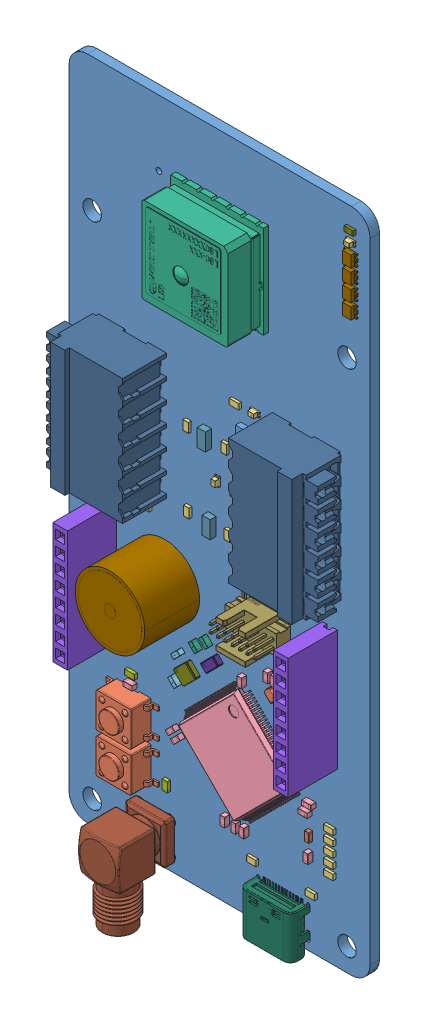
SolidWorks assembly Main_Board_1_1, configuration Default. Lengths in mm.
Overall size (70 133 15.95).
128 component instances, 40 part files, 0 mates.
Components (placement in the parent):
- Main_Board_1_1_BOARD-1: Main_Board_1_1_BOARD [Default] at origin size (52 115 1.63)
- BMP581_CMP-048-000000-2-1: BMP581_CMP-048-000000-2 [Default] at (43 50.5 0.0203) x (-0.707107 -0.707107 0) z (0 0 -1) size (2 2 0.8)
- BMP581_CMP-048-000000-2-2: BMP581_CMP-048-000000-2 [Default] at (45.5 45.5 1.6065) x (0.707107 -0.707107 0) z (0 0 1) size (2 2 0.8)
- RESC1609X50X30ML8T20_CMP-009-00185-4-1: RESC1609X50X30ML8T20_CMP-009-00185-4 [Default] at (40.25 53.25 0.0203) x (0 1 0) z (0 0 -1) size (1.65 0.95 0.5)
- RESC1609X50X30ML8T20_CMP-009-00185-4-2: RESC1609X50X30ML8T20_CMP-009-00185-4 [Default] at (47.5 49 0.0203) x (0 1 0) z (0 0 -1) size (1.65 0.95 0.5)
- RESC1609X50X30ML8T20_CMP-009-00185-4-3: RESC1609X50X30ML8T20_CMP-009-00185-4 [Default] at (41.5 53.25 0.0203) x (0 1 0) z (0 0 -1) size (1.65 0.95 0.5)
- RESC1609X50X30ML8T20_CMP-009-00185-4-4: RESC1609X50X30ML8T20_CMP-009-00185-4 [Default] at (46.0298 49.0299 0.0203) x (0 1 0) z (0 0 -1) size (1.65 0.95 0.5)
- RESC1609X50X30ML8T20_CMP-009-00185-4-5: RESC1609X50X30ML8T20_CMP-009-00185-4 [Default] at (45.25 53.25 0.0203) x (0 1 0) z (0 0 -1) size (1.65 0.95 0.5)
- RESC1609X50X30ML8T20_CMP-009-00185-4-6: RESC1609X50X30ML8T20_CMP-009-00185-4 [Default] at (41.75 47.25 0.0203) x (-1 0 0) z (0 0 -1) size (1.65 0.95 0.5)
- RESC1609X50X30ML8T20_CMP-009-00185-4-7: RESC1609X50X30ML8T20_CMP-009-00185-4 [Default] at (22.375 64 1.6065) x (-1 0 0) z (0 0 1) size (1.65 0.95 0.5)
- RESC1609X50X30ML8T20_CMP-009-00185-4-8: RESC1609X50X30ML8T20_CMP-009-00185-4 [Default] at (23.5 62.75 1.6065) x (-1 0 0) z (0 0 1) size (1.65 0.95 0.5)
- RESC1609X50X30ML8T20_CMP-009-00185-4-9: RESC1609X50X30ML8T20_CMP-009-00185-4 [Default] at (38.337 62.824 0.0203) x (1 0 0) z (0 0 -1) size (1.65 0.95 0.5)
- RESC1609X50X30ML8T20_CMP-009-00185-4-10: RESC1609X50X30ML8T20_CMP-009-00185-4 [Default] at (36.322 28.829 0.0203) x (0 1 0) z (0 0 -1) size (1.65 0.95 0.5)
- RESC1609X50X30ML8T20_CMP-009-00185-4-11: RESC1609X50X30ML8T20_CMP-009-00185-4 [Default] at (39.263 48.645 1.6065) x (0 1 0) z (0 0 1) size (1.65 0.95 0.5)
- RESC1609X50X30ML8T20_CMP-009-00185-4-12: RESC1609X50X30ML8T20_CMP-009-00185-4 [Default] at (44.5 38.75 0.0203) x (1 0 0) z (0 0 -1) size (1.65 0.95 0.5)
- RESC1609X50X30ML8T20_CMP-009-00185-4-13: RESC1609X50X30ML8T20_CMP-009-00185-4 [Default] at (40.914 48.645 1.6065) x (0 1 0) z (0 0 1) size (1.65 0.95 0.5)
- RESC1609X50X30ML8T20_CMP-009-00185-4-14: RESC1609X50X30ML8T20_CMP-009-00185-4 [Default] at (30 78.25 0.0203) x (0 1 0) z (0 0 -1) size (1.65 0.95 0.5)
- RESC1609X50X30ML8T20_CMP-009-00185-4-15: RESC1609X50X30ML8T20_CMP-009-00185-4 [Default] at (32.25 81 0.0203) x (-1 0 0) z (0 0 -1) size (1.65 0.95 0.5)
- RESC1609X50X30ML8T20_CMP-009-00185-4-16: RESC1609X50X30ML8T20_CMP-009-00185-4 [Default] at (35 78.25 0.0203) x (0 -1 0) z (0 0 -1) size (1.65 0.95 0.5)
- RESC1609X50X30ML8T20_CMP-009-00185-4-17: RESC1609X50X30ML8T20_CMP-009-00185-4 [Default] at (41 73.5 0.0203) x (0 1 0) z (0 0 -1) size (1.65 0.95 0.5)
- RESC1609X50X30ML8T20_CMP-009-00185-4-18: RESC1609X50X30ML8T20_CMP-009-00185-4 [Default] at (34.5 73 0.0203) x (0 -1 0) z (0 0 -1) size (1.65 0.95 0.5)
- RESC1609X50X30ML8T20_CMP-009-00185-4-19: RESC1609X50X30ML8T20_CMP-009-00185-4 [Default] at (36.25 73 0.0203) x (0 1 0) z (0 0 -1) size (1.65 0.95 0.5)
- RESC1609X50X30ML8T20_CMP-009-00185-4-20: RESC1609X50X30ML8T20_CMP-009-00185-4 [Default] at (30.6372 78.25 1.6065) x (0 -1 0) z (0 0 1) size (1.65 0.95 0.5)
- RESC1609X50X30ML8T20_CMP-009-00185-4-21: RESC1609X50X30ML8T20_CMP-009-00185-4 [Default] at (30.75 65.5 1.6065) x (0 -1 0) z (0 0 1) size (1.65 0.95 0.5)
- RESC1609X50X30ML8T20_CMP-009-00185-4-22: RESC1609X50X30ML8T20_CMP-009-00185-4 [Default] at (39.75 77.1815 1.6065) x (0 1 0) z (0 0 1) size (1.65 0.95 0.5)
- RESC1609X50X30ML8T20_CMP-009-00185-4-23: RESC1609X50X30ML8T20_CMP-009-00185-4 [Default] at (39.75 65.5 1.6065) x (0 1 0) z (0 0 1) size (1.65 0.95 0.5)
- RESC1609X50X30ML8T20_CMP-009-00185-4-24: RESC1609X50X30ML8T20_CMP-009-00185-4 [Default] at (37.1957 78.25 1.6065) x (0 -1 0) z (0 0 1) size (1.65 0.95 0.5)
- RESC1609X50X30ML8T20_CMP-009-00185-4-25: RESC1609X50X30ML8T20_CMP-009-00185-4 [Default] at (37.75 65.5 1.6065) x (0 -1 0) z (0 0 1) size (1.65 0.95 0.5)
- RESC1609X50X30ML8T20_CMP-009-00185-4-26: RESC1609X50X30ML8T20_CMP-009-00185-4 [Default] at (38.9707 85.75 1.6065) x (-1 0 0) z (0 0 1) size (1.65 0.95 0.5)
- RESC1609X50X30ML8T20_CMP-009-00185-4-27: RESC1609X50X30ML8T20_CMP-009-00185-4 [Default] at (38.75 72.5 1.6065) x (0 1 0) z (0 0 1) size (1.65 0.95 0.5)
- RESC1609X50X30ML8T20_CMP-009-00185-4-28: RESC1609X50X30ML8T20_CMP-009-00185-4 [Default] at (55.245 23.495 1.6065) size (1.65 0.95 0.5)
- RESC1609X50X30ML8T20_CMP-009-00185-4-29: RESC1609X50X30ML8T20_CMP-009-00185-4 [Default] at (55.245 25.1777 1.6065) size (1.65 0.95 0.5)
- RESC1609X50X30ML8T20_CMP-009-00185-4-30: RESC1609X50X30ML8T20_CMP-009-00185-4 [Default] at (55.245 26.8605 1.6065) size (1.65 0.95 0.5)
- RESC1609X50X30ML8T20_CMP-009-00185-4-31: RESC1609X50X30ML8T20_CMP-009-00185-4 [Default] at (55.245 28.5433 1.6065) size (1.65 0.95 0.5)
- RESC1609X50X30ML8T20_CMP-009-00185-4-32: RESC1609X50X30ML8T20_CMP-009-00185-4 [Default] at (55.245 30.226 1.6065) size (1.65 0.95 0.5)
- RESC1609X50X30ML8T20_CMP-009-00185-4-33: RESC1609X50X30ML8T20_CMP-009-00185-4 [Default] at (52.07 18.923 1.6065) size (1.65 0.95 0.5)
- RESC1609X50X30ML8T20_CMP-009-00185-4-34: RESC1609X50X30ML8T20_CMP-009-00185-4 [Default] at (41.91 18.923 1.6065) x (-1 0 0) z (0 0 1) size (1.65 0.95 0.5)
- RESC1609X50X30ML8T20_CMP-009-00185-4-35: RESC1609X50X30ML8T20_CMP-009-00185-4 [Default] at (52.125 55.125 1.6065) x (-1 0 0) z (0 0 1) size (1.65 0.95 0.5)
- RESC1609X50X30ML8T20_CMP-009-00185-4-36: RESC1609X50X30ML8T20_CMP-009-00185-4 [Default] at (36.5 54.5 0.0203) x (0 1 0) z (0 0 -1) size (1.65 0.95 0.5)
- RESC1609X50X30ML8T20_CMP-009-00185-4-37: RESC1609X50X30ML8T20_CMP-009-00185-4 [Default] at (38 54.5 0.0203) x (0 1 0) z (0 0 -1) size (1.65 0.95 0.5)
- RESC1609X50X30ML8T20_CMP-009-00185-4-38: RESC1609X50X30ML8T20_CMP-009-00185-4 [Default] at (52.125 57.375 1.6065) x (-1 0 0) z (0 0 1) size (1.65 0.95 0.5)
- RESC1609X50X30ML8T20_CMP-009-00185-4-39: RESC1609X50X30ML8T20_CMP-009-00185-4 [Default] at (41.75 45.75 0.0203) x (1 0 0) z (0 0 -1) size (1.65 0.95 0.5)
- RESC1609X50X30ML8T20_CMP-009-00185-4-40: RESC1609X50X30ML8T20_CMP-009-00185-4 [Default] at (41.75 44.25 0.0203) x (1 0 0) z (0 0 -1) size (1.65 0.95 0.5)
- FP-0603-L_1_6_0_15-W_0_81-IPC_C_CMP-001-00088-6-1: FP-0603-L_1_6_0_15-W_0_81-IPC_C_CMP-001-00088-6 [Default] at (42.75 53.25 0.0203) x (0 -1 0) z (0 0 -1) size (1.65 0.86 0.94)
- FP-0603-L_1_6_0_15-W_0_81-IPC_C_CMP-001-00088-6-2: FP-0603-L_1_6_0_15-W_0_81-IPC_C_CMP-001-00088-6 [Default] at (46 48 1.6065) x (0 -1 0) z (0 0 1) size (1.65 0.86 0.94)
- FP-0603-L_1_6_0_15-W_0_81-IPC_C_CMP-001-00088-6-3: FP-0603-L_1_6_0_15-W_0_81-IPC_C_CMP-001-00088-6 [Default] at (44 53.25 0.0203) x (0 -1 0) z (0 0 -1) size (1.65 0.86 0.94)
- FP-0603-L_1_6_0_15-W_0_81-IPC_C_CMP-001-00088-6-4: FP-0603-L_1_6_0_15-W_0_81-IPC_C_CMP-001-00088-6 [Default] at (44.75 48 1.6065) x (0 -1 0) z (0 0 1) size (1.65 0.86 0.94)
- FP-0603-L_1_6_0_15-W_0_81-IPC_C_CMP-001-00088-6-5: FP-0603-L_1_6_0_15-W_0_81-IPC_C_CMP-001-00088-6 [Default] at (29.21 30.861 1.6065) x (0.707107 0.707107 0) z (0 0 1) size (1.65 0.86 0.94)
- FP-0603-L_1_6_0_15-W_0_81-IPC_C_CMP-001-00088-6-6: FP-0603-L_1_6_0_15-W_0_81-IPC_C_CMP-001-00088-6 [Default] at (32.25 75.75 0.0203) x (1 0 0) z (0 0 -1) size (1.65 0.86 0.94)
- FP-0603-L_1_6_0_15-W_0_81-IPC_C_CMP-001-00088-6-7: FP-0603-L_1_6_0_15-W_0_81-IPC_C_CMP-001-00088-6 [Default] at (44 78.5 0.0203) x (0 1 0) z (0 0 -1) size (1.65 0.86 0.94)
- FP-0603-L_1_6_0_15-W_0_81-IPC_C_CMP-001-00088-6-8: FP-0603-L_1_6_0_15-W_0_81-IPC_C_CMP-001-00088-6 [Default] at (42.5 73.5 0.0203) x (0 -1 0) z (0 0 -1) size (1.65 0.86 0.94)
- FP-0603-L_1_6_0_15-W_0_81-IPC_C_CMP-001-00088-6-9: FP-0603-L_1_6_0_15-W_0_81-IPC_C_CMP-001-00088-6 [Default] at (44 73.5 0.0203) x (0 -1 0) z (0 0 -1) size (1.65 0.86 0.94)
- FP-0603-L_1_6_0_15-W_0_81-IPC_C_CMP-001-00088-6-10: FP-0603-L_1_6_0_15-W_0_81-IPC_C_CMP-001-00088-6 [Default] at (42.5 78.5 0.0203) x (0 1 0) z (0 0 -1) size (1.65 0.86 0.94)
- FP-0603-L_1_6_0_15-W_0_81-IPC_C_CMP-001-00088-6-11: FP-0603-L_1_6_0_15-W_0_81-IPC_C_CMP-001-00088-6 [Default] at (38.375 39.625 0.0203) x (0 -1 0) z (0 0 -1) size (1.65 0.86 0.94)
- FP-0603-L_1_6_0_15-W_0_81-IPC_C_CMP-001-00088-6-12: FP-0603-L_1_6_0_15-W_0_81-IPC_C_CMP-001-00088-6 [Default] at (40.25 45 1.6065) x (0 -1 0) z (0 0 1) size (1.65 0.86 0.94)
- FP-0603-L_1_6_0_15-W_0_81-IPC_C_CMP-001-00088-6-13: FP-0603-L_1_6_0_15-W_0_81-IPC_C_CMP-001-00088-6 [Default] at (51.816 32.385 1.6065) x (-1 0 0) z (0 0 1) size (1.65 0.86 0.94)
- FP-0603-L_1_6_0_15-W_0_81-IPC_C_CMP-001-00088-6-14: FP-0603-L_1_6_0_15-W_0_81-IPC_C_CMP-001-00088-6 [Default] at (37.125 39.625 0.0203) x (0 -1 0) z (0 0 -1) size (1.65 0.86 0.94)
- FP-0603-L_1_6_0_15-W_0_81-IPC_C_CMP-001-00088-6-15: FP-0603-L_1_6_0_15-W_0_81-IPC_C_CMP-001-00088-6 [Default] at (28.321 31.75 1.6065) x (0.707107 0.707107 0) z (0 0 1) size (1.65 0.86 0.94)
- FP-0603-L_1_6_0_15-W_0_81-IPC_C_CMP-001-00088-6-16: FP-0603-L_1_6_0_15-W_0_81-IPC_C_CMP-001-00088-6 [Default] at (40.64 22.733 1.6065) x (0 1 0) z (0 0 1) size (1.65 0.86 0.94)
- FP-0603-L_1_6_0_15-W_0_81-IPC_C_CMP-001-00088-6-17: FP-0603-L_1_6_0_15-W_0_81-IPC_C_CMP-001-00088-6 [Default] at (39.243 22.733 1.6065) x (0 1 0) z (0 0 1) size (1.65 0.86 0.94)
- FP-0603-L_1_6_0_15-W_0_81-IPC_C_CMP-001-00088-6-18: FP-0603-L_1_6_0_15-W_0_81-IPC_C_CMP-001-00088-6 [Default] at (20.955 34.798 1.6065) size (1.65 0.86 0.94)
- FP-0603-L_1_6_0_15-W_0_81-IPC_C_CMP-001-00088-6-19: FP-0603-L_1_6_0_15-W_0_81-IPC_C_CMP-001-00088-6 [Default] at (37.338 22.733 1.6065) x (0 -1 0) z (0 0 1) size (1.65 0.86 0.94)
- FP-0603-L_1_6_0_15-W_0_81-IPC_C_CMP-001-00088-6-20: FP-0603-L_1_6_0_15-W_0_81-IPC_C_CMP-001-00088-6 [Default] at (51.181 30.861 1.6065) size (1.65 0.86 0.94)
- FP-0603-L_1_6_0_15-W_0_81-IPC_C_CMP-001-00088-6-21: FP-0603-L_1_6_0_15-W_0_81-IPC_C_CMP-001-00088-6 [Default] at (31.496 39.624 0.0203) x (0 -1 0) z (0 0 -1) size (1.65 0.86 0.94)
- FP-0603-L_1_6_0_15-W_0_81-IPC_C_CMP-001-00088-6-22: FP-0603-L_1_6_0_15-W_0_81-IPC_C_CMP-001-00088-6 [Default] at (30.353 39.624 0.0203) x (0 -1 0) z (0 0 -1) size (1.65 0.86 0.94)
- FP-0603-L_1_6_0_15-W_0_81-IPC_C_CMP-001-00088-6-23: FP-0603-L_1_6_0_15-W_0_81-IPC_C_CMP-001-00088-6 [Default] at (51.689 24.4251 1.6065) x (0 -1 0) z (0 0 1) size (1.65 0.86 0.94)
- FP-0603-L_1_6_0_15-W_0_81-IPC_C_CMP-001-00088-6-24: FP-0603-L_1_6_0_15-W_0_81-IPC_C_CMP-001-00088-6 [Default] at (34.5 92.75 0.0203) x (0 -1 0) z (0 0 -1) size (1.65 0.86 0.94)
- FP-0603-L_1_6_0_15-W_0_81-IPC_C_CMP-001-00088-6-25: FP-0603-L_1_6_0_15-W_0_81-IPC_C_CMP-001-00088-6 [Default] at (39.988 60.411 0.0203) x (0 1 0) z (0 0 -1) size (1.65 0.86 0.94)
- FP-0603-L_1_6_0_15-W_0_81-IPC_C_CMP-001-00088-6-26: FP-0603-L_1_6_0_15-W_0_81-IPC_C_CMP-001-00088-6 [Default] at (33.511 61.3 0.0203) x (0 1 0) z (0 0 -1) size (1.65 0.86 0.94)
- FP-0603-L_1_6_0_15-W_0_81-IPC_C_CMP-001-00088-6-27: FP-0603-L_1_6_0_15-W_0_81-IPC_C_CMP-001-00088-6 [Default] at (35.67 62.57 0.0203) x (-1 0 0) z (0 0 -1) size (1.65 0.86 0.94)
- FP-0603-L_1_6_0_15-W_0_81-IPC_C_CMP-001-00088-6-28: FP-0603-L_1_6_0_15-W_0_81-IPC_C_CMP-001-00088-6 [Default] at (33.782 37.592 0.0203) x (1 0 0) z (0 0 -1) size (1.65 0.86 0.94)
- FP-0603-L_1_6_0_15-W_0_81-IPC_C_CMP-001-00088-2-1: FP-0603-L_1_6_0_15-W_0_81-IPC_C_CMP-001-00088-2 [Default] at (37 117.5 0.0203) x (1 0 0) z (0 0 -1) size (1.6 0.81 0.9)
- FP-0603-L_1_6_0_15-W_0_81-IPC_C_CMP-001-00088-2-2: FP-0603-L_1_6_0_15-W_0_81-IPC_C_CMP-001-00088-2 [Default] at (37 96.75 0.0203) x (-1 0 0) z (0 0 -1) size (1.6 0.81 0.9)
- FP-0603-L_1_6_0_15-W_0_81-IPC_C_CMP-001-00088-2-3: FP-0603-L_1_6_0_15-W_0_81-IPC_C_CMP-001-00088-2 [Default] at (37 101.75 0.0203) x (-1 0 0) z (0 0 -1) size (1.6 0.81 0.9)
- FP-0603-L_1_6_0_15-W_0_81-IPC_C_CMP-001-00088-2-4: FP-0603-L_1_6_0_15-W_0_81-IPC_C_CMP-001-00088-2 [Default] at (42 96.75 0.0203) x (1 0 0) z (0 0 -1) size (1.6 0.81 0.9)
- FP-0603-L_1_6_0_15-W_0_81-IPC_C_CMP-001-00088-2-5: FP-0603-L_1_6_0_15-W_0_81-IPC_C_CMP-001-00088-2 [Default] at (42 101.75 0.0203) x (1 0 0) z (0 0 -1) size (1.6 0.81 0.9)
- QUEC-L80-M39-12_V_CMP-021-00008-3-1: QUEC-L80-M39-12_V_CMP-021-00008-3 [Default] at (36.48 107 1.6065) x (0 1 0) z (0 0 1) size (16 16 6.95)
- RESC1608X55X25ML10T15_CMP-009-00177-3-1: RESC1608X55X25ML10T15_CMP-009-00177-3 [Default] at (37.3293 68.1458 0.0203) x (1 0 0) z (0 0 -1) size (1.7 0.9 0.55)
- RESC1608X55X25ML10T15_CMP-009-00177-3-2: RESC1608X55X25ML10T15_CMP-009-00177-3 [Default] at (27.051 22.733 1.6065) x (0 -1 0) z (0 0 1) size (1.7 0.9 0.55)
- RESC1608X55X25ML10T15_CMP-009-00177-3-3: RESC1608X55X25ML10T15_CMP-009-00177-3 [Default] at (34.5 88.6457 0.0203) x (0 1 0) z (0 0 -1) size (1.7 0.9 0.55)
- RESC1608X55X25ML10T15_CMP-009-00177-3-4: RESC1608X55X25ML10T15_CMP-009-00177-3 [Default] at (20.955 36.322 1.6065) x (-1 0 0) z (0 0 1) size (1.7 0.9 0.55)
- AO-SOT-23-3L_V_CMP-013-00037-1-1: AO-SOT-23-3L_V_CMP-013-00037-1 [Default] at (33.25 69.3457 0.0203) x (0 1 0) z (0 0 -1) size (3 3.1 1.25)
- LED_WS2812-2020_CMP-002-000000-1-1: LED_WS2812-2020_CMP-002-000000-1 [Default] at (58.778 112.3103 1.6065) x (-1 0 0) z (0 0 1) size (2.2 2 0.84)
- LED_WS2812-2020_CMP-002-000000-1-2: LED_WS2812-2020_CMP-002-000000-1 [Default] at (58.778 109.728 1.6065) x (-1 0 0) z (0 0 1) size (2.2 2 0.84)
- LED_WS2812-2020_CMP-002-000000-1-3: LED_WS2812-2020_CMP-002-000000-1 [Default] at (58.778 117.475 1.6065) x (-1 0 0) z (0 0 1) size (2.2 2 0.84)
- LED_WS2812-2020_CMP-002-000000-1-4: LED_WS2812-2020_CMP-002-000000-1 [Default] at (58.778 114.8927 1.6065) x (-1 0 0) z (0 0 1) size (2.2 2 0.84)
- FP-S8411-45R-MFG_CMP-002-00079-1-1: FP-S8411-45R-MFG_CMP-002-00079-1 [Default] at (25.527 110.165 0.0203) x (-1 0 0) z (0 0 -1) size (14.75 19.2 5.45)
- MCC-SOD-123FL_V_CMP-004-00034-1-1: MCC-SOD-123FL_V_CMP-004-00034-1 [Default] at (29.4186 89.9257 0.0203) x (0 1 0) z (0 0 -1) size (3.7 1.9 1.2)
- MCC-SOD-123FL_V_CMP-004-00034-1-2: MCC-SOD-123FL_V_CMP-004-00034-1 [Default] at (31.8228 90.158 0.0203) x (0 1 0) z (0 0 -1) size (3.7 1.9 1.2)
- FP-FTSH-107-01-F-DV-K-MFG_CMP-002-00087-1-1: FP-FTSH-107-01-F-DV-K-MFG_CMP-002-00087-1 [Default] at (44.25 55.75 1.6065) x (-1 0 0) z (0 0 1) size (8.97 5.87 6.44)
- FP-SOT23-IPC_C_CMP-013-00038-1-1: FP-SOT23-IPC_C_CMP-013-00038-1 [Default] at (26.924 48.006 0.0203) x (-1 0 0) z (0 0 -1) size (2.82 2.9 1.25)
- SOT95P245X110-5N_CMP-011-00013-1-1: SOT95P245X110-5N_CMP-011-00013-1 [Default] at (33.9165 78.2 1.6065) size (1.4 3 1.05)
- SOT95P245X110-5N_CMP-011-00013-1-2: SOT95P245X110-5N_CMP-011-00013-1 [Default] at (34.75 65.5 1.6065) size (1.4 3 1.05)
- THRMC1608X95N_CMP-038-000000-2-1: THRMC1608X95N_CMP-038-000000-2 [Default] at (29.8107 70.6457 0.0203) x (1 0 0) z (0 0 -1) size (1.6 0.8 0.45)
- FP-CRCW0603-e3-IPC_C_0603WAF220JT5E-2-1: FP-CRCW0603-e3-IPC_C_0603WAF220JT5E-2 [Default] at (58.75 121.5 1.6065) x (-1 0 0) z (0 0 1) size (1.55 0.85 0.5)
- SOT95P230X110-3N_CMP-013-000004-1-1: SOT95P230X110-3N_CMP-013-000004-1 [Default] at (37.5 77.75 0.0203) x (0 -1 0) z (0 0 -1) size (2.4 2.9 0.95)
- SSM6J507NULF_CMP-013-000003-10-1: SSM6J507NULF_CMP-013-000003-10 [Default] at (38.75 73.675 0.0203) x (0 -1 0) z (0 0 -1) size (2 2.22 0.9)
- AON7544_CMP-089-000000-2-1: AON7544_CMP-089-000000-2 [Default] at (41.225 81.7657 1.6065) x (0 -1 0) z (0 0 1) size (3.13 3.23 1)
- AON7544_CMP-089-000000-2-2: AON7544_CMP-089-000000-2 [Default] at (41.39 69.25 1.6065) x (0 -1 0) z (0 0 1) size (3.13 3.23 1)
- FP-BLM18-0_15-0_1-t0_6-IPC_B_CMP-006-00021-1-1: FP-BLM18-0_15-0_1-t0_6-IPC_B_CMP-006-00021-1 [Default] at (51.689 27.4731 1.6065) x (0 1 0) z (0 0 1) size (1.6 0.8 0.7)
- FP-BLM18-0_15-0_1-t0_6-IPC_B_CMP-006-00021-1-2: FP-BLM18-0_15-0_1-t0_6-IPC_B_CMP-006-00021-1 [Default] at (29.591 37.719 0.0203) x (-1 0 0) z (0 0 -1) size (1.6 0.8 0.7)
- FP-LTST-C190GKT-MFG_CMP-00026-00001-1-1: FP-LTST-C190GKT-MFG_CMP-00026-00001-1 [Default] at (58.75 119.75 1.6065) size (1.6 0.8 0.9)
- FP-LTST-C190GKT-MFG_CMP-00026-00001-1-2: FP-LTST-C190GKT-MFG_CMP-00026-00001-1 [Default] at (42.25 86 1.6065) x (-1 0 0) z (0 0 1) size (1.6 0.8 0.9)
- FP-LTST-C190GKT-MFG_CMP-00026-00001-1-3: FP-LTST-C190GKT-MFG_CMP-00026-00001-1 [Default] at (35.75 72.5 1.6065) x (0 -1 0) z (0 0 1) size (1.6 0.8 0.9)
- MCC-SOD123_V_CMP-004-00005-3-1: MCC-SOD123_V_CMP-004-00005-3 [Default] at (41.5 76 0.0203) x (1 0 0) z (0 0 -1) size (2.7 1.6 1.35)
- FP-CL10-IPC_B_CMP-001-00087-1-1: FP-CL10-IPC_B_CMP-001-00087-1 [Default] at (28.702 39.243 1.6065) x (-0.707107 0.707107 0) z (0 0 1) size (1.6 0.8 0.9)
- FP-CL10-IPC_B_CMP-001-00087-1-2: FP-CL10-IPC_B_CMP-001-00087-1 [Default] at (29.21 43.561 1.6065) x (-0.707107 -0.707107 0) z (0 0 1) size (1.6 0.8 0.9)
- FP-CL10-IPC_B_CMP-001-00086-2-1: FP-CL10-IPC_B_CMP-001-00086-2 [Default] at (32.258 46.228 1.6065) x (-0.707107 0.707107 0) z (0 0 1) size (1.6 0.8 0.9)
- FP-CL10-IPC_B_CMP-001-00086-2-2: FP-CL10-IPC_B_CMP-001-00086-2 [Default] at (34.036 47.752 1.6065) x (-0.707107 0.707107 0) z (0 0 1) size (1.6 0.8 0.9)
- CAPPM3528X210N_CMP-054-000000-2-1: CAPPM3528X210N_CMP-054-000000-2 [Default] at (43.5 65.6458 0.0203) x (0 1 0) z (0 0 -1) size (3.5 2.85 2.1)
- SLIN-PPPC081LFBN-RC_V_CMP-002-00028-2-1: SLIN-PPPC081LFBN-RC_V_CMP-002-00028-2 [Default] at (16.95 50 1.6065) x (0 -1 0) z (0 0 1) size (20.82 2.54 11.7)
- SLIN-PPPC081LFBN-RC_V_CMP-002-00028-2-2: SLIN-PPPC081LFBN-RC_V_CMP-002-00028-2 [Default] at (55.05 50 1.6065) x (0 -1 0) z (0 0 1) size (20.82 2.54 11.7)
- KXG1203C_CMP-059-000000-1-1: KXG1203C_CMP-059-000000-1 [Default] at (26.543 53.086 1.6065) x (0 1 0) z (0 0 1) size (12 12 14)
- SHDR12W80P700X350_2X6_2170X1400X850P_CMP-062-000000-2-1: SHDR12W80P700X350_2X6_2170X1400X850P_CMP-062-000000-2 [Default] at (53.75 67.75 1.6065) x (0 1 0) z (0 0 1) size (21.7 14.3 12)
- SHDR12W80P700X350_2X6_2170X1400X850P_CMP-062-000000-2-2: SHDR12W80P700X350_2X6_2170X1400X850P_CMP-062-000000-2 [Default] at (18.25 85 1.6065) x (0 -1 0) z (0 0 1) size (21.7 14.3 12)
- PCBSMAFRAHT_CMP-070-000000-2-1: PCBSMAFRAHT_CMP-070-000000-2 [Default] at (24.857 14.951 1.6065) x (-1 0 0) z (0 0 1) size (9.21 15.6 13.8)
- FP-BNO085-MFG_CMP-010-00028-1-1: FP-BNO085-MFG_CMP-010-00028-1 [Default] at (36.5 59 0.0203) x (-1 0 0) z (0 0 -1) size (3.8 5.2 1.18)
- SOT65P210X110-5N_CMP-064-000000-3-1: SOT65P210X110-5N_CMP-064-000000-3 [Default] at (32.25 78.5 0.0203) x (0 -1 0) z (0 0 -1) size (2.12 2 1.1)
- LoRa-CC68-868-TCXO-Footprint-1_CMP-00025-00003-3-1: LoRa-CC68-868-TCXO-Footprint-1_CMP-00025-00003-3 [Default] at (25.146 27.94 0.0203) x (-1 0 0) z (0 0 -1) size (16 16 2.1)
- VALCON_CSP-USC16-TR_CMP-042-000000-3-1: VALCON_CSP-USC16-TR_CMP-042-000000-3 [Default] at (47 16.891 1.6065) size (8.94 7.75 4.26)
- FP-NX3225GA-MFG_CMP-003-00030-1-1: FP-NX3225GA-MFG_CMP-003-00030-1 [Default] at (30.734 41.402 1.6065) x (-0.707107 -0.707107 0) z (0 0 1) size (3.21 2.51 0.9)
- FP-NX3215SA-MFG_CMP-003-00031-1-1: FP-NX3215SA-MFG_CMP-003-00031-1 [Default] at (35.052 44.958 1.6065) x (-0.707107 -0.707107 0) z (0 0 1) size (3.21 1.51 0.9)
- SOIC127P790X216-8N_CMP-040-000000-2-1: SOIC127P790X216-8N_CMP-040-000000-2 [Default] at (39.878 35.687 0.0203) x (-1 0 0) z (0 0 -1) size (7.9 5.28 2.16)
- D0008A_L_CMP-019-00052-1-1: D0008A_L_CMP-019-00052-1 [Default] at (39.009 90.1617 0.0203) x (1 0 0) z (0 0 -1) size (6 4.9 1.63)
- CKCP-PTS645S_V_CMP-011-00016-1-1: CKCP-PTS645S_V_CMP-011-00016-1 [Default] at (21.131 24.257 1.6065) x (-1 0 0) z (0 0 1) size (9 6 4.3)
- CKCP-PTS645S_V_CMP-011-00016-1-2: CKCP-PTS645S_V_CMP-011-00016-1 [Default] at (21.131 31.115 1.6065) x (-1 0 0) z (0 0 1) size (9 6 4.3)
- MOLX-473521001_V_CMP-002-00077-1-1: MOLX-473521001_V_CMP-002-00077-1 [Default] at (48.7 25 0.0203) x (0 -1 0) z (0 0 -1) size (14.1 15.2 1.89)
- QFP50P1600X1600X160-100N_CMP-028-000000-1-1: QFP50P1600X1600X160-100N_CMP-028-000000-1 [Default] at (40 34 1.6065) x (0.707107 -0.707107 0) z (0 0 1) size (16 16 1.6)
